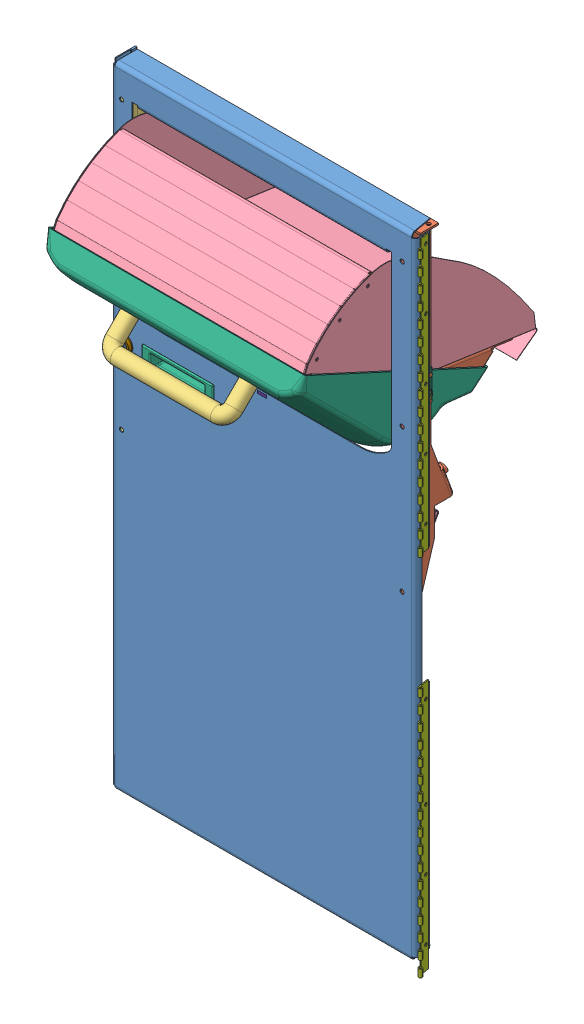
SolidWorks assembly BB3_Assy_Meca_3D_Devidoir_sujet, configuration Défaut. Lengths in mm.
Overall size (899.17 1279.45 776.24).
99 component instances, 62 part files, 6 mates.
Components (placement in the parent):
- BB3_Porte-1: BB3_Porte [Défaut] at (-537.6945 281.2509 1236.9474) x (-1 0 0) z (0 0 -1) size (899.17 1120.24 468.39)
  - Porte_Devant-1: Porte_Devant [Défaut] at (265.4153 -39.6917 -280.2063) size (521.6 1080.12 53)
  - Porte_Plaque_Support_Devidoir_Droite-1: Porte_Plaque_Support_Devidoir_Droite [Défaut] at (-239.7055 206.7117 47.939) x (0.939693 -0.321394 0.116978) z (0.34202 0.883022 -0.321394) size (245.58 270.63 576.7)
  - Porte_Plaque_Support_Devidoir_Gauche-1: Porte_Plaque_Support_Devidoir_Gauche [Défaut] at (253.7381 206.7117 47.939) x (-0.939693 -0.321394 0.116978) z (0.34202 -0.883022 0.321394) size (235.72 270.63 576.7)
  - Porte_Plaque_Support_Devidoir_Centre-1: Porte_Plaque_Support_Devidoir_Centre [Défaut] at (7.0162 30.6943 16.6558) x (0 -0.258819 0.965926) z (-1 0 0) size (85.71 18.5 445.2)
  - Porte_Poignee_Arriere-1: Porte_Poignee_Arriere [Défaut] at (150.1174 92.5415 -24.8999) x (1 0 0) z (0 1 0) size (121.4 25.4 64.3)
  - Porte_Poignee_Devant-1: Porte_Poignee_Devant [Défaut] at (150.1174 85.2415 -2.5999) x (1 0 0) z (0 1 0) size (122.99 27.13 46.9)
  - Porte_Charniere-1: Porte_Charniere [Défaut] at (-277.2955 -54.1847 3.3348) x (-0.173648 0 -0.984808) z (0 1 0) size (21.77 6 1092)
  - Porte_Serrure_Cle-1: Porte_Serrure_Cle [Défaut] at (242.4153 102.2755 6.859) x (0 0 1) z (1 0 0) size (41.58 38.56 38.97)
    - Porte_Serrure_Ressort-1: Porte_Serrure_Ressort [Défaut] at (-1.4058 10.243 9.1044) x (0 0 -1) z (1 0 0) size (21.49 4.59 4.57)
    - Porte_Serrure_Support-1: Porte_Serrure_Support [Défaut] at (-26.6815 11.1833 12.473) x (-1 0 0) z (0 -1 0) size (41.46 28.7 28.7)
    - Porte_Serrure_Insert_Cle-1: Porte_Serrure_Insert_Cle [Défaut] at (26.379 -212.8643 14.6) x (-1 0 0) z (0 0 -1) size (23.33 15.95 15.95)
    - Porte_Serrure_Ecrou_Hex-1: Porte_Serrure_Ecrou_Hex [Défaut] at (-26.3115 -31.157 8.2014) x (0 0 1) z (-1 0 0) size (33 28.58 4.76)
    - Porte_Serrure_Rondelle_Ecrou-1: Porte_Serrure_Rondelle_Ecrou [Défaut] at (-31.074 17.7899 -9.8703) x (0 0.096744 0.995309) z (-1 0 0) size (35.31 35.31 0.64)
    - Porte_Serrure_Came-1: Porte_Serrure_Came [Défaut] at (-18.246 14.5659 16.3878) x (0 -1 0) z (1 0 0) size (12.45 12.01 13.54)
    - Porte_Serrure_Pene-1: Porte_Serrure_Pene [Défaut] at (1.0072 5.2825 -10.1896) x (0 -0.999973 -0.007317) z (-1 0 0) size (16.91 23.47 9.63)
  - Porte_Support_Devidoir-1: Porte_Support_Devidoir [Défaut] at (-219.5828 230.7583 15.6101) x (0 0 1) z (1 0 0) size (44 50 2)
  - Porte_Support_Devidoir-2: Porte_Support_Devidoir [Défaut] at (233.6153 230.7583 15.6101) x (0 0 1) z (-1 0 0) size (44 50 2)
  - Porte_Coussinet-1: Porte_Coussinet [Défaut] at (-217.0588 230.7583 12.6101) x (0 0.383049 -0.923728) z (0 0.923728 0.383049) size (28.27 19.05 28.27)
  - Porte_Coussinet-2: Porte_Coussinet [Défaut] at (231.0913 230.7583 12.6101) x (0 0.383049 0.923728) z (0 0.923728 -0.383049) size (28.27 19.05 28.27)
  - Porte_Plaque_Support_Devidoir_Gauche_simulation-1: Porte_Plaque_Support_Devidoir_Gauche_simulation [Défaut] at (214.5427 74.8366 69.753) x (-1 0 0) z (0 0.34202 0.939693) size (15.52 15.52 7.76)
  - Porte_Plaque_Support_Devidoir_Gauche_simulation-2: Porte_Plaque_Support_Devidoir_Gauche_simulation [Défaut] at (7.0173 130.9233 -18.7399) x (1 0 0) z (0 1 0) size (15.52 15.52 7.76)
- BB3_Dévidoir_allégé-1: BB3_Dévidoir_allégé [Défaut] at (-284.0469 510.2249 1235.5381) x (-0.795138 -0.086285 -0.600259) z (-0.363434 0.86018 0.357779) size (642 556.94 573.94)
  - HopperRollRod_Rev3-1: HopperRollRod_Rev3 [Default] at (155.8236 65.6237 286.0909) x (0.795138 0.485459 0.363434) z (-0.19783 0.774165 -0.601275) size (428.62 9.53 9.53)
  - PEM-FH-0420-20-1: PEM-FH-0420-20 [Default] at (393.3249 56.2024 61.1725) x (0.795138 0.485459 0.363434) z (-0.606428 0.636526 0.476529) size (8.56 31.75 8.56)
  - PEM-FH-0420-20-2: PEM-FH-0420-20 [Default] at (231.7529 -42.443 -12.6774) x (0.795138 0.485459 0.363434) z (-0.606428 0.636526 0.476529) size (8.56 31.75 8.56)
  - DoorShield_Rev2-2: DoorShield_Rev2 [Default] at (302.6515 19.535 28.9751) x (-0.795138 -0.485459 -0.363434) z (0.606428 -0.636526 -0.476529) size (434.07 74.67 214.39)
  - HANDLE_MC_1435A43-1: HANDLE_MC_1435A43 [Default] at (121.4778 196.7862 188.5909) x (-0.795138 -0.485459 -0.363434) z (-0.363434 0.861227 -0.355251) size (228.6 25.4 88.9)
  - HopperBase_Rev1-2: HopperBase_Rev1 [Default] at (116.9003 195.0314 200.9498) x (-0.795138 -0.485459 -0.363434) z (-0.363434 0.861227 -0.355251) size (431.8 386.04 237.96)
  - HopperRod_Rev3-3: HopperRod_Rev3 [Default] at (213.8333 117.6327 92.2617) x (0.795138 0.485459 0.363434) z (-0.363434 -0.098284 0.926421) size (482.6 19.05 19.05)
  - HopperSkin_Rev1-2: HopperSkin_Rev1 [Default] at (213.8331 117.6327 92.2616) x (-0.795138 -0.485459 -0.363434) z (-0.172906 0.755914 -0.631424) size (450.64 354.33 119.73)
- BB3_Chassis-1: BB3_Chassis [Défaut] at (-560.1006 692.3812 848.6503) size (671.41 1282.03 663.93) (hidden)
  - TopCrossmember_Rev2-1: TopCrossmember_Rev2 [Default] at (20.5473 102.5902 0) size (635 86.99 210.82)
  - TopCrossMotorBrkt_Rev3-1: TopCrossMotorBrkt_Rev3 [Défaut] at (-101.9976 61.051 0) size (152.4 200.54 205.51)
  - Moto_Reducteur_011_562_1_216-1: Moto_Reducteur_011_562_1_216 [Default] at (192.9322 74.2423 -36.8146) x (0 -0.000019 -1) z (-1 0 0) size (114.3 226.4 239.81)
  - TopCrossBearingBrkt_Rev1-1: TopCrossBearingBrkt_Rev1 [Défaut] at (-246.0257 61.051 0) size (25.4 73.66 205.51)
  - TopCrossBearingBrkt_Rev1-2: TopCrossBearingBrkt_Rev1 [Défaut] at (287.1203 61.051 0) x (-1 0 0) z (0 0 -1) size (25.4 73.66 205.51)
  - Chassis_Coussinet-1: Chassis_Coussinet [Default] at (-247.5497 60.2788 -36.8146) x (0 -0.995993 0.089436) z (0 0.089436 0.995993) size (28.27 19.05 28.27)
  - Chassis_Coussinet-2: Chassis_Coussinet [Default] at (288.6443 60.2788 -36.8146) x (0 0.997938 0.064185) z (0 -0.064185 0.997938) size (28.27 19.05 28.27)
  - Chassis_Support_Moteur-1: Chassis_Support_Moteur [Défaut] at (-296.9017 100.6288 0.0002) x (0 0 1) z (0 1 0) size (205.51 54 1127)
  - Chassis_Support_Moteur-2: Chassis_Support_Moteur [Défaut] at (337.9963 100.6288 0.0002) x (0 0 -1) z (0 1 0) size (205.51 54 1127)
  - Chassis_Panneau_Arriere-2: Chassis_Panneau_Arriere [Défaut] at (20.5983 -479.4712 -246.619) x (0 0 1) z (0 1 0) size (164.98 667 1155.29)
  - Chassis_Support_Batterie-2: Chassis_Support_Batterie [Défaut] at (20.5983 -270.8192 -242.544) x (0 0 1) z (-1 0 0) size (116.32 446 529)
  - Chassis_Support_Moteur_Devant_Gauche-2: Chassis_Support_Moteur_Devant_Gauche [Défaut] at (-249.8894 -442.8187 130.7585) x (0 0 -1) z (0 1 0) size (329.85 66 1105)
  - Chassis_Positionnement_Emetteur_Recepteur_Gauche-2: Chassis_Positionnement_Emetteur_Recepteur_Gauche [Défaut] at (-222.4622 -381.8185 156.8606) x (1 0 0) z (0 -1 0) size (22.1 48.5 273)
  - Chassis_Support_Moteur_Devant_Droite-1: Chassis_Support_Moteur_Devant_Droite [Défaut] at (290.9839 -442.8187 130.7585) x (0 0 -1) z (0 -1 0) size (329.85 66 1105)
  - Chassis_Positionnement_Emetteur_Recepteur_Droite-1: Chassis_Positionnement_Emetteur_Recepteur_Droite [Défaut] at (263.5568 -381.8185 156.8606) x (-1 0 0) z (0 1 0) size (22.1 48.5 273)
  - Chassis_Support_Pignon_bas-1: Chassis_Support_Pignon_bas [Défaut] at (305.4963 -865.3715 -39.8528) x (-1 0 0) z (0 0 1) size (35.2 151.29 95)
  - Chassis_Axe_Pignon_Bas-1: Chassis_Axe_Pignon_Bas [Défaut] at (340.9963 -816.3715 -39.8528) x (-1 0 0) z (0 -0.052233 -0.998635) size (48.6 15.9 15.9)
  - Chassis_Goupille_Axe_Pignon_bas-1: Chassis_Goupille_Axe_Pignon_bas [Défaut] at (300.5463 -817.6251 -63.8201) x (0 0.052233 0.998635) z (1 0 0) size (60.5 23 3)
  - Chassis_Support_Pignon_bas-2: Chassis_Support_Pignon_bas [Défaut] at (-264.4017 -865.3715 -39.8528) x (1 0 0) z (0 0 -1) size (35.2 151.29 95)
  - Chassis_Axe_Pignon_Bas-2: Chassis_Axe_Pignon_Bas [Défaut] at (-299.9017 -816.3715 -39.8528) x (1 0 0) z (0 0.31653 0.948583) size (48.6 15.9 15.9)
  - Chassis_Goupille_Axe_Pignon_bas-2: Chassis_Goupille_Axe_Pignon_bas [Défaut] at (-259.4517 -808.7748 -17.0869) x (0 -0.31653 -0.948583) z (1 0 0) size (60.5 23 3)
  - Chassis_Plaque_Haute-1: Chassis_Plaque_Haute [Défaut] at (20.4963 92.768 412.6062) x (0 0 -1) z (1 0 0) size (278.51 354.1 562.7)
  - Chassis_Renfort-1: Chassis_Renfort [Défaut] at (20.5463 -1018.8712 0.0002) x (0 0 1) z (-1 0 0) size (199.51 39 641)
  - Chassis_Charniere_Photovoltaique-1: Chassis_Charniere_Photovoltaique [Défaut] at (20.5983 134.4053 -220.1468) x (0 0 -1) z (1 0 0) size (21.77 6 520)
  - Chassis_Equerre_Haute-1: Chassis_Equerre_Haute [Défaut] at (-246.1446 112.2812 81.6782) x (1 0 0.000001) z (-0.000001 0 1) size (44 37.45 648)
  - Chassis_Equerre_Haute-2: Chassis_Equerre_Haute [Défaut] at (287.2893 112.2812 81.6751) x (-1 0 -0.000168) z (0.000168 0 -1) size (44 37.45 648)
  - Chassis_Repose_Bac_Dechets-1: Chassis_Repose_Bac_Dechets [Défaut] at (20.4963 -992.8728 80.2436) x (0 -0.000001 1) z (-1 0 0) size (641.73 77 529)
  - Chassis_Semelle-1: Chassis_Semelle [Défaut] at (20.4963 -1034.3925 80.4561) x (1 0 0) z (0 -0.000001 1) size (404.15 56 558)
  - Chassis_Repose_Pied-1: Chassis_Repose_Pied [Défaut] at (-187.0037 -1049.3185 336.4561) x (1 0 0) z (0 -0.000001 1) size (94 52.5 63.3)
  - Chassis_Repose_Pied-2: Chassis_Repose_Pied [Défaut] at (-187.0037 -1049.3182 -175.5439) x (1 0 0) z (0 -0.000001 1) size (94 52.5 63.3)
  - Chassis_Repose_Pied-3: Chassis_Repose_Pied [Défaut] at (227.9963 -1049.3182 -175.5439) x (1 0 0) z (0 -0.000001 1) size (94 52.5 63.3)
  - Chassis_Repose_Pied-4: Chassis_Repose_Pied [Défaut] at (227.9963 -1049.3185 336.4561) x (1 0 0) z (0 -0.000001 1) size (94 52.5 63.3)
  - Chassis_Repose_Pied_Insert-1: Chassis_Repose_Pied_Insert [Défaut] at (-187.0037 -1050.3185 336.4561) x (0 1 0.000001) z (0.428959 -0.000001 0.903324) size (14.3 17.5 17.5)
  - Chassis_Repose_Pied_Insert-2: Chassis_Repose_Pied_Insert [Défaut] at (227.9963 -1050.3185 336.4561) x (0 1 0.000001) z (0.384049 -0.000001 0.923313) size (14.3 17.5 17.5)
  - Chassis_Repose_Pied_Insert-3: Chassis_Repose_Pied_Insert [Défaut] at (227.9963 -1050.3182 -175.5439) x (0 1 0.000001) z (-0.000001 -0.000001 1) size (14.3 17.5 17.5)
  - Chassis_Repose_Pied_Insert-4: Chassis_Repose_Pied_Insert [Défaut] at (-187.0037 -1050.3182 -175.5439) x (0 1 0.000001) z (-0.000001 -0.000001 1) size (14.3 17.5 17.5)
  - Chassis_Repose_Pied_Insert-5: Chassis_Repose_Pied_Insert [Défaut] at (-114.0037 -995.8185 336.4561) x (0 -1 -0.000001) z (0.798225 0 0.602359) size (14.3 17.5 17.5)
  - Chassis_Repose_Pied_Insert-6: Chassis_Repose_Pied_Insert [Défaut] at (154.9963 -995.8185 336.4561) x (0 -1 -0.000001) z (0.000001 -0.000001 1) size (14.3 17.5 17.5)
  - Chassis_Repose_Pied_Insert-7: Chassis_Repose_Pied_Insert [Défaut] at (-114.0037 -995.8182 -175.5439) x (0 -1 -0.000001) z (0.000001 -0.000001 1) size (14.3 17.5 17.5)
  - Chassis_Repose_Pied_Insert-8: Chassis_Repose_Pied_Insert [Défaut] at (154.9963 -995.8182 -175.5439) x (0 -1 -0.000001) z (0.000001 -0.000001 1) size (14.3 17.5 17.5)
  - Chassis_Dessous_Avant_Porte-1: Chassis_Dessous_Avant_Porte [Défaut] at (20.4963 -992.8728 80.2436) x (0 -0.000001 1) z (-1 0 0) size (98 53.79 536)
  - Chassis_Serrure-1: Chassis_Serrure [Défaut] at (-243.4017 -382.964 366.4072) x (1 0 0) z (0 1 0) size (10.5 63.82 216)
  - Chassis_Equerre_Face-1: Chassis_Equerre_Face [Défaut] at (20.4963 111.0096 411.9878) x (0 0 1) z (-1 0 0) size (32.2 41.42 529)
  - Chassis_Charniere_Support_Moteur_Devant_Droite-1: Chassis_Charniere_Support_Moteur_Devant_Droite [Défaut] at (260.2718 -465.3185 388.412) x (0 0 1) z (0 -1 0) size (21.77 6 1066)
  - Chassis_Serrure_Cle-1: Chassis_Serrure_Cle [Défaut] at (-191.3537 126.1269 363.7894) x (0 1 0) z (-1 0 0) size (41.58 38.56 38.97)
    - Chassis_Serrure_Came-1: Chassis_Serrure_Came [Défaut] at (-18.246 14.5659 16.3878) x (0 -1 0) z (1 0 0) size (12.45 12.01 13.54)
    - Chassis_Serrure_Rondelle_Ecrou-1: Chassis_Serrure_Rondelle_Ecrou [Défaut] at (-31.074 17.7899 -9.8703) x (0 0.096744 0.995309) z (-1 0 0) size (35.31 35.31 0.64)
    - Chassis_Serrure_Ecrou_Hex-1: Chassis_Serrure_Ecrou_Hex [Défaut] at (-26.3115 -31.157 8.2014) x (0 0 1) z (-1 0 0) size (33 28.58 4.76)
    - Chassis_Serrure_Insert_Cle-1: Chassis_Serrure_Insert_Cle [Défaut] at (26.379 -212.8643 14.6) x (-1 0 0) z (0 0 -1) size (23.33 15.95 15.95)
    - Chassis_Serrure_Support-1: Chassis_Serrure_Support [Défaut] at (-26.6815 11.1833 12.473) x (-1 0 0) z (0 -1 0) size (41.46 28.7 28.7)
    - Chassis_Serrure_Ressort-1: Chassis_Serrure_Ressort [Défaut] at (-1.4058 10.243 9.1044) x (0 0 -1) z (1 0 0) size (21.49 4.59 4.57)
    - Chassis_Serrure_Pene-1: Chassis_Serrure_Pene [Défaut] at (1.0072 5.2825 -10.1896) x (0 -0.999973 -0.007317) z (-1 0 0) size (16.91 23.47 9.63)
  - Chassis_Serrure_Cle-2: Chassis_Serrure_Cle [Défaut] at (232.3463 126.1269 341.4229) x (0 1 0) z (1 0 0) size (41.58 38.56 38.97)
    - Chassis_Serrure_Came-1: Chassis_Serrure_Came [Défaut] at (-18.246 14.5659 16.3878) x (0 -1 0) z (1 0 0) size (12.45 12.01 13.54)
    - Chassis_Serrure_Rondelle_Ecrou-1: Chassis_Serrure_Rondelle_Ecrou [Défaut] at (-31.074 17.7899 -9.8703) x (0 0.096744 0.995309) z (-1 0 0) size (35.31 35.31 0.64)
    - Chassis_Serrure_Ecrou_Hex-1: Chassis_Serrure_Ecrou_Hex [Défaut] at (-26.3115 -31.157 8.2014) x (0 0 1) z (-1 0 0) size (33 28.58 4.76)
    - Chassis_Serrure_Insert_Cle-1: Chassis_Serrure_Insert_Cle [Défaut] at (26.379 -212.8643 14.6) x (-1 0 0) z (0 0 -1) size (23.33 15.95 15.95)
    - Chassis_Serrure_Support-1: Chassis_Serrure_Support [Défaut] at (-26.6815 11.1833 12.473) x (-1 0 0) z (0 -1 0) size (41.46 28.7 28.7)
    - Chassis_Serrure_Ressort-1: Chassis_Serrure_Ressort [Défaut] at (-1.4058 10.243 9.1044) x (0 0 -1) z (1 0 0) size (21.49 4.59 4.57)
    - Chassis_Serrure_Pene-1: Chassis_Serrure_Pene [Défaut] at (1.0072 5.2825 -10.1896) x (0 -0.999973 -0.007317) z (-1 0 0) size (16.91 23.47 9.63)
  - Tombstone_Rev1-1: Tombstone_Rev1 [Default] at (288.5894 129.5652 81.0473) x (1 0 0.000168) z (-0.000168 0 1) size (22.23 105.62 654.05)
  - Tombstone_Rev1-2: Tombstone_Rev1 [Default] at (-247.4446 129.5652 82.3062) x (-1 0 -0.000001) z (0.000001 0 -1) size (22.23 105.62 654.05)
  - SideSkin_Rev1-1: SideSkin_Rev1 [Default] at (-317.3073 -1045.6118 82.3061) x (-1 0 -0.000001) z (0.000001 0 -1) size (69.87 1274.83 660.4) (hidden)
  - SideSkin_Rev1-2: SideSkin_Rev1 [Default] at (358.4521 -1045.6118 81.059) x (1 0 0.000168) z (-0.000168 0 1) size (69.87 1274.83 660.4)
  - Chassis_Interieur_Cache_Chaine-1: Chassis_Interieur_Cache_Chaine [Défaut] at (-242.9017 -763.8184 0) x (0 -0.000001 1) z (-1 0 0) size (249 989 21) (hidden)
  - Chassis_Interieur_Cache_Chaine-2: Chassis_Interieur_Cache_Chaine [Défaut] at (283.9963 -763.8185 0.0002) x (0 0 -1) z (1 0 0) size (249 989 21)
  - Chassis_Bac_Dechets-1: Chassis_Bac_Dechets [Défaut] at (19.5983 -711.9931 65.1059) x (-1 0 0) z (0 0.000001 -1) size (517 387.96 620.45) (hidden)
Mates (geometry in assembly coordinates):
- Coaxiale1: concentric anti-aligned: cylinder of BB3_Porte-1/Porte_Coussinet-2 through (-207.3688 512.0092 1745.0493) axis (0.211815 0 0.97731) radius 9.6139; cylinder of BB3_Dévidoir_allégé-1/HopperRod_Rev3-3 through (-203.7202 512.0092 1761.8835) axis (-0.211815 0 -0.97731) radius 9.525
- Coïncidente1: coincident aligned: plane of BB3_Porte-1/Porte_Plaque_Support_Devidoir_Centre-1; plane of BB3_Dévidoir_allégé-1/HANDLE_MC_1435A43-1
- Angle1: planar angle = 0.785398 rad aligned: plane of BB3_Porte-1/Porte_Devant-1; plane of BB3_Dévidoir_allégé-1/HopperSkin_Rev1-2
- Coaxiale2: concentric anti-aligned: cylinder of BB3_Porte-1/Porte_Charniere-1 through (-278.1043 227.0662 1258.3064) axis (0 1 0) radius 1.5; cylinder of BB3_Chassis-1/Chassis_Charniere_Support_Moteur_Devant_Droite-1 through (-278.1043 227.0627 1258.3064) axis (0 -1 0) radius 1.5
- Distance2: distance = 3.54 mm anti-aligned: plane of BB3_Chassis-1/Chassis_Plaque_Haute-1 through (-539.6043 785.1492 1261.2564) normal (0 -1 0); plane of BB3_Porte-1/Porte_Devant-1 through (-249.5567 781.6092 1224.9473) normal (0 1 0)
- Angle2: planar angle = 0 rad aligned: plane of BB3_Porte-1/Porte_Devant-1 through (-249.5567 781.6092 1263.4473) normal (0 0 1); plane of BB3_Chassis-1/Chassis_Support_Moteur_Devant_Gauche-2 through (-804.0023 -364.4899 1259.2564) normal (0 0 1)
